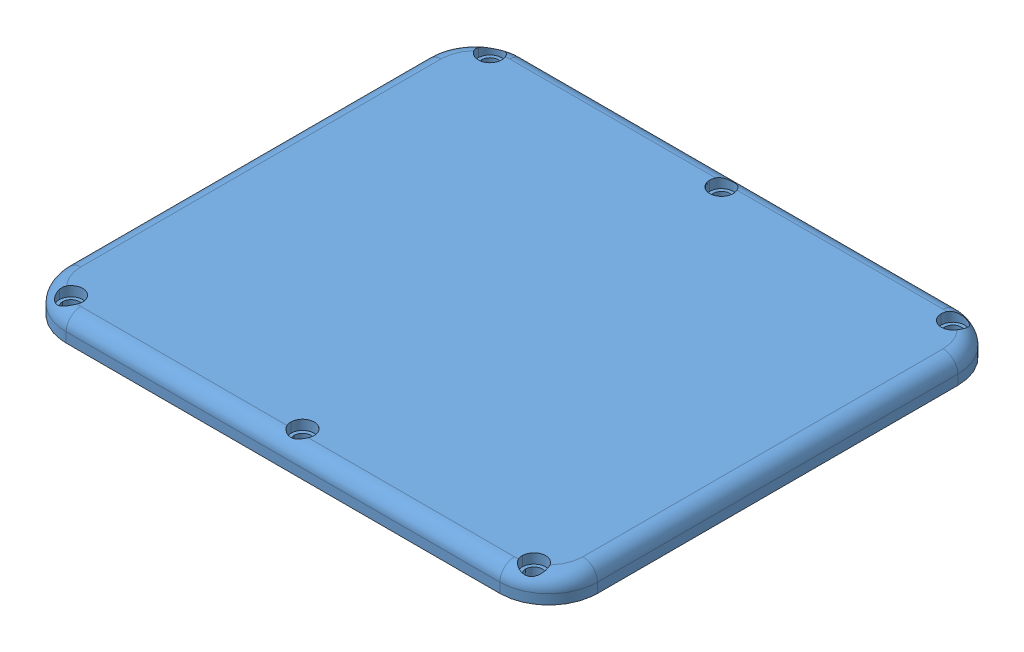
SolidWorks assembly enclosure step, configuration Default. Lengths in mm.
Overall size (108.67 5.02 93.67).
123 component instances, 60 part files, 0 mates.
Components (placement in the parent):
- enclosure step.STEP-1: enclosure step.STEP [Default] at origin size (108.67 110.01 98.74)
  - PCB_Mouser - Copy.step.STEP-1: PCB_Mouser - Copy.step.STEP [Default] at (-12.7572 -8.0885 -81.5279) x (0.000739 0 1) z (0 1 0) size (74.49 49.75 15) (hidden)
    - Board.step.STEP-1: Board.step.STEP [Default] at origin size (74.49 42.98 0.41)
      - Open CASCADE STEP translator 7.5 1.1.1.step.STEP-1: Open CASCADE STEP translator 7.5 1.1.1.step.STEP [Default] at (0 0 -0.4115) size (74.49 42.98 0.41)
    - U1.step.STEP-1: U1.step.STEP [Default] at origin size (6.5 7 1.8)
      - 5987470688.step.STEP-1: 5987470688.step.STEP [Default] at (33.655 29.7184 0) x (0 -1 0) z (0 0 1) size (7 6.5 1.8)
        - Body.step.STEP-1: Body.step.STEP [Default] at origin size (3.5 6.5 1.74)
        - PinsArrayL.step.STEP-1: PinsArrayL.step.STEP [Default] at origin size (1.75 5.35 1.18)
        - FilletPinR.step.STEP-1: FilletPinR.step.STEP [Default] at origin size (1.75 3 1.18)
    - C2.step.STEP-1: C2.step.STEP [Default] at origin size (1.55 3.2 1.8)
      - 5987470768.step.STEP-1: 5987470768.step.STEP [Default] at (31.1762 37.4434 0) x (0 1 0) z (0 0 1) size (3.2 1.55 1.8)
        - Body-0.step.STEP-1: Body-0.step.STEP [Default] at origin size (3 1.55 1.7)
        - FilletPin1.step.STEP-1: FilletPin1.step.STEP [Default] at origin size (0.75 1.2 0.86)
        - FilletPin2.step.STEP-1: FilletPin2.step.STEP [Default] at origin size (0.85 1.2 0.86)
    - C1.step.STEP-1: C1.step.STEP [Default] at origin size (1.55 3.2 1.8)
      - 5987470768.step.STEP-1: 5987470768.step.STEP [Default] at (36.0172 37.418 0) x (0 1 0) z (0 0 1) size (3.2 1.55 1.8)
        - Body-0.step.STEP-1: Body-0.step.STEP [Default] at origin size (3 1.55 1.7)
        - FilletPin1.step.STEP-1: FilletPin1.step.STEP [Default] at origin size (0.75 1.2 0.86)
        - FilletPin2.step.STEP-1: FilletPin2.step.STEP [Default] at origin size (0.85 1.2 0.86)
    - C4.step.STEP-1: C4.step.STEP [Default] at origin size (1.6 0.8 0.95)
      - 5987472768.step.STEP-1: 5987472768.step.STEP [Default] at (25.7 16 0) x (-1 0 0) z (0 0 1) size (1.6 0.8 0.95)
        - Fillet1.step.STEP-1: Fillet1.step.STEP [Default] at origin size (0.35 0.8 0.95)
        - Fillet2.step.STEP-1: Fillet2.step.STEP [Default] at origin size (0.35 0.8 0.95)
        - body2.step.STEP-1: body2.step.STEP [Default] at origin size (0.9 0.78 0.93)
    - C6.step.STEP-1: C6.step.STEP [Default] at origin size (0.8 1.6 0.95)
      - 5987470208.step.STEP-1: 5987470208.step.STEP [Default] at (61 3 0) x (0 -1 0) z (0 0 1) size (1.6 0.8 0.95)
        - Fillet1-1.step.STEP-1: Fillet1-1.step.STEP [Default] at origin size (0.35 0.8 0.95)
        - Fillet2-2.step.STEP-1: Fillet2-2.step.STEP [Default] at origin size (0.35 0.8 0.95)
        - body2-3.step.STEP-1: body2-3.step.STEP [Default] at origin size (0.9 0.78 0.93)
    - C5.step.STEP-1: C5.step.STEP [Default] at origin size (0.8 1.6 0.95)
      - 5987470208.step.STEP-1: 5987470208.step.STEP [Default] at (8 4 0) x (0 -1 0) z (0 0 1) size (1.6 0.8 0.95)
        - Fillet1-1.step.STEP-1: Fillet1-1.step.STEP [Default] at origin size (0.35 0.8 0.95)
        - Fillet2-2.step.STEP-1: Fillet2-2.step.STEP [Default] at origin size (0.35 0.8 0.95)
        - body2-3.step.STEP-1: body2-3.step.STEP [Default] at origin size (0.9 0.78 0.93)
    - D1.step.STEP-1: D1.step.STEP [Default] at origin size (2.18 0.8 0.8)
      - 5987472288.step.STEP-1: 5987472288.step.STEP [Default] at (24.35 26.25 0) x (0 -1 0) z (0 0 1) size (0.8 2.18 0.8)
        - Body-4.step.STEP-1: Body-4.step.STEP [Default] at (0 0 0.1) size (0.8 1.2 0.7)
        - Pins.step.STEP-1: Pins.step.STEP [Default] at origin size (0.68 2.18 0.1)
    - J1.step.STEP-1: J1.step.STEP [Default] at origin size (7.4 5.75 10.4)
      - 5987472128.step.STEP-1: 5987472128.step.STEP [Default] at (61 39.5 0) x (-1 0 0) z (0 0 1) size (7.4 5.75 10.4)
        - Body-5.step.STEP-1: Body-5.step.STEP [Default] at origin size (7.4 5.75 7)
        - LeadsArray.step.STEP-1: LeadsArray.step.STEP [Default] at origin size (3.14 0.64 10.4)
    - R11.step.STEP-1: R11.step.STEP [Default] at origin size (1.25 2 0.5)
      - 5987471968.step.STEP-1: 5987471968.step.STEP [Default] at (18.4 11.5 0.25) x (0 1 0) z (1 0 0) size (2 0.5 1.25)
    - R10.step.STEP-1: R10.step.STEP [Default] at origin size (1.25 2 0.5)
      - 5987471888.step.STEP-1: 5987471888.step.STEP [Default] at (25.4 5.7 0.25) x (0 -1 0) z (-1 0 0) size (2 0.5 1.25)
    - R8.step.STEP-1: R8.step.STEP [Default] at origin size (1.25 2 0.5)
      - 5987471968.step.STEP-1: 5987471968.step.STEP [Default] at (25.4 9.45 0.25) x (0 1 0) z (1 0 0) size (2 0.5 1.25)
    - R7.step.STEP-1: R7.step.STEP [Default] at origin size (1.25 2 0.5)
      - 5987471888.step.STEP-1: 5987471888.step.STEP [Default] at (25.4 13.2 0.25) x (0 -1 0) z (-1 0 0) size (2 0.5 1.25)
    - R5.step.STEP-1: R5.step.STEP [Default] at origin size (2 1.25 0.5)
      - 5987471808.step.STEP-1: 5987471808.step.STEP [Default] at (17.85 15.75 0.25) x (1 0 0) z (0 -1 0) size (2 0.5 1.25)
    - R4.step.STEP-1: R4.step.STEP [Default] at origin size (2 1.25 0.5)
      - 5987471808.step.STEP-1: 5987471808.step.STEP [Default] at (23.9 19.5 0.25) x (1 0 0) z (0 -1 0) size (2 0.5 1.25)
    - Q1.step.STEP-1: Q1.step.STEP [Default] at origin size (2.4 2.9 0.95)
      - 5987471568.step.STEP-1: 5987471568.step.STEP [Default] at (17.04 18.67 -1.16) x (0 1 0) z (1 0 0) size (2.9 0.95 2.4)
        - SOT23 lower body.step.STEP-1: SOT23 lower body.step.STEP [Default] at (2.782 1.6068 2.7442) x (-1 0 0) z (0 0 1) size (2.9 0.4 1.27)
        - SOT23 Lead.step.STEP-1: SOT23 Lead.step.STEP [Default] at (1.122 1.4868 2.7295) x (0 0 -1) z (1 0 0) size (0.58 0.45 0.42)
        - SOT23 Lead.step.STEP-2: SOT23 Lead.step.STEP [Default] at (2.492 1.4868 1.489) x (0 0 1) z (-1 0 0) size (0.58 0.45 0.42)
        - SOT23 Lead.step.STEP-3: SOT23 Lead.step.STEP [Default] at (0.592 1.4868 1.489) x (0 0 1) z (-1 0 0) size (0.58 0.45 0.42)
        - SOT23 Upper body.step.STEP-1: SOT23 Upper body.step.STEP [Default] at (-0.118 1.6068 2.7442) size (2.9 0.5 1.27)
    - U2.step.STEP-1: U2.step.STEP [Default] at origin size (16 24 3.1)
      - 5987472528.step.STEP-1: 5987472528.step.STEP [Default] at (38.9 5.25 1.6) x (-1 0 0) z (0 1 0) size (16 3.1 24)
    - S2.step.STEP-1: S2.step.STEP [Default] at origin size (5.2 6.4 1.55)
      - 5987472208.step.STEP-1: 5987472208.step.STEP [Default] at (70.15 9 0.55) x (1 0 0) z (0 -1 0) size (5.2 1.55 6.4)
    - S1.step.STEP-1: S1.step.STEP [Default] at origin size (6.4 5.2 1.55)
      - 6089891264.step.STEP-1: 6089891264.step.STEP [Default] at (16.4 4.25 0.55) x (0 1 0) z (1 0 0) size (5.2 1.55 6.4)
    - R13.step.STEP-1: R13.step.STEP [Default] at origin size (1.25 2 0.5)
      - 5987471888.step.STEP-1: 5987471888.step.STEP [Default] at (52.15 3.2 0.25) x (0 -1 0) z (-1 0 0) size (2 0.5 1.25)
    - R12.step.STEP-1: R12.step.STEP [Default] at origin size (1.25 2 0.5)
      - 5987471968.step.STEP-1: 5987471968.step.STEP [Default] at (52.15 7.25 0.25) x (0 1 0) z (1 0 0) size (2 0.5 1.25)
    - R9.step.STEP-1: R9.step.STEP [Default] at origin size (1.25 2 0.5)
      - 5987471888.step.STEP-1: 5987471888.step.STEP [Default] at (52.15 11.7 0.25) x (0 -1 0) z (-1 0 0) size (2 0.5 1.25)
    - R6.step.STEP-1: R6.step.STEP [Default] at origin size (2 1.25 0.5)
      - 5987470848.step.STEP-1: 5987470848.step.STEP [Default] at (52.4 21.25 0.25) x (-1 0 0) z (0 1 0) size (2 0.5 1.25)
    - R3.step.STEP-1: R3.step.STEP [Default] at origin size (2 1.25 0.5)
      - 6089890704.step.STEP-1: 6089890704.step.STEP [Default] at (44 29.75 0.25) x (1 0 0) z (0 -1 0) size (2 0.5 1.25)
    - R2.step.STEP-1: R2.step.STEP [Default] at origin size (2 1.25 0.5)
      - 6089890704.step.STEP-1: 6089890704.step.STEP [Default] at (49 29.75 0.25) x (1 0 0) z (0 -1 0) size (2 0.5 1.25)
    - R1.step.STEP-1: R1.step.STEP [Default] at origin size (1.25 2 0.6)
      - 6089895904.step.STEP-1: 6089895904.step.STEP [Default] at (39.5 31.705 0) x (0 -1 0) z (-1 0 0) size (2 0.6 1.25)
    - LS1.step.STEP-1: LS1.step.STEP [Default] at origin size (12 12 15)
      - CUI_DEVICES_CMI-1295-0585T.step.STEP-1: CUI_DEVICES_CMI-1295-0585T.step.STEP [Default] at (18.346 33.654 1.2) x (-1 0 0) z (0 1 0) size (12 15 12)
    - J5.step.STEP-1: J5.step.STEP [Default] at origin size (15.75 2.54 11.71)
      - 6089888224.step.STEP-1: 6089888224.step.STEP [Default] at (37.96 21.75 0) x (-1 0 0) z (0 1 0) size (15.75 11.71 2.54)
    - J4.step.STEP-1: J4.step.STEP [Default] at origin size (5.1 10 11.6)
      - 110990030--3DModel-STEP-56544.step.STEP-1: 110990030--3DModel-STEP-56544.step.STEP [Default] at (69.9 20 1) x (0 1 0) z (1 0 0) size (10 11.6 5.1)
    - J3.step.STEP-1: J3.step.STEP [Default] at origin size (2.54 20.32 11.54)
      - 5987472048.step.STEP-1: 5987472048.step.STEP [Default] at (2.65 12.13 0) x (0 1 0) z (0 0 1) size (20.32 2.54 11.54)
        - Body-6.step.STEP-1: Body-6.step.STEP [Default] at origin size (20.32 2.54 2.54)
        - LeadsArray-7.step.STEP-1: LeadsArray-7.step.STEP [Default] at origin size (18.42 0.64 11.54)
    - J2.step.STEP-1: J2.step.STEP [Default] at origin size (5.75 7.4 10.4)
      - 5987472848.step.STEP-1: 5987472848.step.STEP [Default] at (70.5 31 0) x (0 1 0) z (0 0 1) size (7.4 5.75 10.4)
        - Body-8.step.STEP-1: Body-8.step.STEP [Default] at origin size (7.4 5.75 7)
        - LeadsArray-9.step.STEP-1: LeadsArray-9.step.STEP [Default] at origin size (3.14 0.64 10.4)
    - C3.step.STEP-1: C3.step.STEP [Default] at origin size (2.01 1.52 1.25)
      - 0805YD106KAT4A.step.STEP-1: 0805YD106KAT4A.step.STEP [Default] at (52.263 15.238 0.6) size (2.01 1.52 1.25)
  - TP4056_Charging_Module_Type_C.step.STEP-1: TP4056_Charging_Module_Type_C.step.STEP [Default] at (-26.991 -8.5 -75.0631) x (0 0 -1) z (0 1 0) size (29.3 17.4 4.14) (hidden)
    - board.step.STEP-1: board.step.STEP [Default] at origin size (28.3 17.4 1.5)
    - USB_Type_C_Connector.step.STEP-1: USB_Type_C_Connector.step.STEP [Default] at (15.15 0 2.82) x (0 1 0) z (0 0 1) size (8.42 7.39 2.79)
    - 8205A_2045.step.STEP-1: 8205A_2045.step.STEP [Default] at (-6.45 2.6 1.6) x (0 1 0) z (0 0 1) size (7.5 3 1.2)
    - DW01-P.step.STEP-1: DW01-P.step.STEP [Default] at (-6.45 -3.9 1.6) x (0 1 0) z (0 0 1) size (2.8 2.9 1.35)
    - small1005_smd_resistor.step.STEP-1: small1005_smd_resistor.step.STEP [Default] at (-3.9 -7.2 1.6) x (0 1 0) z (0 0 1) size (1 0.5 0.35)
    - small1005_smd_resistor (1).step.STEP-1: small1005_smd_resistor (1).step.STEP [Default] at (-3.9 5.8 1.6) x (0 1 0) z (0 0 1) size (1 0.5 0.35)
    - small1005_smd_capacitor.step.STEP-1: small1005_smd_capacitor.step.STEP [Default] at (-3.9 -1.2 1.6) x (0 1 0) z (0 0 1) size (1 0.5 0.35)
    - smd_capacitor.step.STEP-1: smd_capacitor.step.STEP [Default] at (-2.225 -1.2 1.6) size (0.85 1.6 0.8)
    - SOP-8_4056E.step.STEP-1: SOP-8_4056E.step.STEP [Default] at (2.3 0.75 1.65) x (-1 0 0) z (0 0 1) size (4.9 6.01 1.69)
    - small1005_smd_resistor.step.STEP-2: small1005_smd_resistor.step.STEP [Default] at (3.35 5.95 1.5) size (1 0.5 0.35)
    - solder_dot_round.step.STEP-1: solder_dot_round.step.STEP [Default] at (1.35 5.95 1.5) size (1 1 0.5)
    - solder_dot_round (1).step.STEP-1: solder_dot_round (1).step.STEP [Default] at (-0.15 5.95 1.5) size (1 1 0.5)
    - solder_dot_round (2).step.STEP-1: solder_dot_round (2).step.STEP [Default] at (6 4 1.5) size (1 1 0.5)
    - solder_dot_round (3).step.STEP-1: solder_dot_round (3).step.STEP [Default] at (6 2.5 1.5) size (1 1 0.5)
    - small1005_smd_capacitor (1).step.STEP-1: small1005_smd_capacitor (1).step.STEP [Default] at (6 -1 1.5) x (0 1 0) z (0 0 1) size (1 0.5 0.35)
    - LED2.step.STEP-1: LED2.step.STEP [Default] at (5.5 -8 1.5) size (3.94 1 1)
    - LED2 (1).step.STEP-1: LED2 (1).step.STEP [Default] at (0.5 -8 1.5) size (3.94 1 1)
    - small1005_smd_resistor (2).step.STEP-1: small1005_smd_resistor (2).step.STEP [Default] at (9.5 -8 1.5) size (1 0.5 0.35)
    - small1005_smd_resistor (4).step.STEP-1: small1005_smd_resistor (4).step.STEP [Default] at (4 -4.5 1.5) size (1 0.5 0.35)
    - small1005_smd_resistor (4).step.STEP-2: small1005_smd_resistor (4).step.STEP [Default] at (0.5 -4.5 1.5) size (1 0.5 0.35)
    - soldering.step.STEP-1: soldering.step.STEP [Default] at origin size (5.77 9.58 1.01)
  - Part1.STEP-1: Part1.STEP [Default] at origin size (108.67 105 98.74) (hidden)
  - Part3.STEP-1: Part3.STEP [Default] at (0 17.5 0) x (1 0 0) z (0 1 0) size (108.67 93.67 5.02)
  - reader.step.STEP-1: reader.step.STEP [Default] at (43.9782 -2.7241 -11.4324) x (-0.017452 -0.99984 -0.003962) z (0.999848 -0.017452 0) size (40 59 21.11) (hidden)
  - OLED-128x64-0.96.step.STEP-1: OLED-128x64-0.96.step.STEP [Default] at (-52.4107 7.9412 -18.5087) x (0 0 1) z (-0.999848 -0.017452 0) size (26.7 28.27 11) (hidden)
